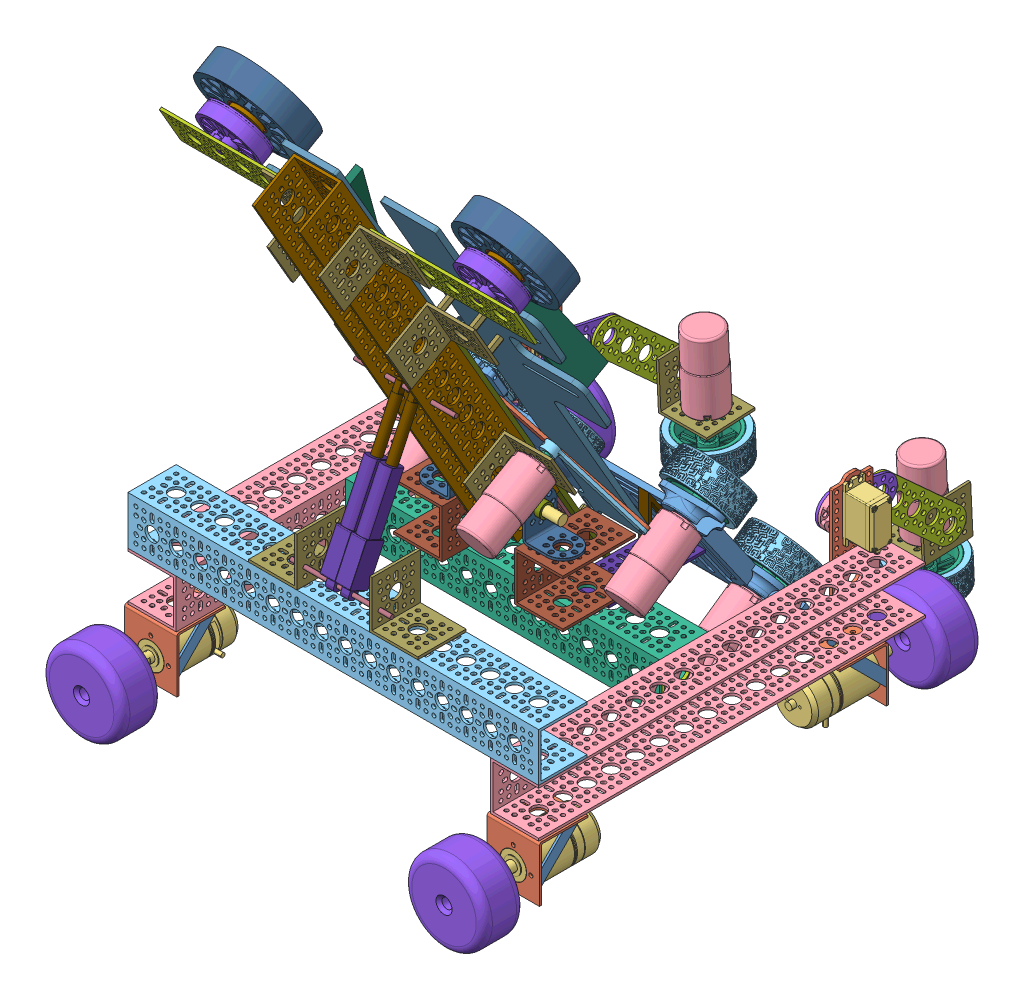
SolidWorks assembly 底座3.0, configuration 默认. Lengths in mm. (continued)
Mates (geometry in assembly coordinates): (continued)
- Concentric428: concentric anti-aligned: cylinder of 连杆02-1 through (57.5295 256.5301 499.31) axis (0 -0.499817 0.866131) radius 1.6; cylinder of 连杆01-5 through (57.5295 253.6311 504.3336) axis (0 0.499817 -0.866131) radius 1.6
- Concentric437: concentric aligned: cylinder of 5孔平板-1 through (85.3414 565.4353 686.9217) axis (0 -0.499817 0.866131) radius 7; cylinder of 发射无刷电机-1 through (85.3414 563.8859 689.6067) axis (0 -0.499817 0.866131) radius 12.5
- Coincident197: coincident anti-aligned: plane of 5孔平板-1 through (-10.6586 580.3085 704.1637) normal (0 0.499817 -0.866131); plane of 发射无刷电机-1 through (85.3414 561.6867 693.4176) normal (0 -0.499817 0.866131)
- Concentric438: concentric aligned: cylinder of 发射无刷电机-1 through (85.3414 578.5805 664.1424) axis (0 -0.499817 0.866131) radius 2; cylinder of 发射法兰-1 through (85.3414 578.0807 665.0086) axis (0 -0.499817 0.866131) radius 2.15
- Tangent7: tangent anti-aligned: plane of 5孔平板-1 through (87.3414 579.2934 694.9187) normal (-1 0 0); cylinder of 发射无刷电机-1 through (86.1414 574.6903 695.8416) axis (0 -0.499817 0.866131) radius 1.2
- Coincident198: coincident anti-aligned: plane of 发射无刷电机-1 through (94.8219 575.055 669.0353) normal (0 0.499817 -0.866131); plane of 发射法兰-1 through (85.3414 575.5816 669.3392) normal (0 -0.499817 0.866131)
- Concentric439: concentric anti-aligned: cylinder of 发射无刷电机-1 through (85.7254 577.7689 677.5287) axis (0 0.499817 -0.866131) radius 1.2; cylinder of 发射法兰-1 through (85.7254 583.2668 668.0013) axis (0 -0.499817 0.866131) radius 1.6
- Concentric440: concentric aligned: cylinder of 发射法兰-1 through (85.3414 581.0796 659.8118) axis (0 -0.499817 0.866131) radius 9.5; cylinder of 摩擦轮-2/摩擦轮.STEP-1/3613-0014-0096 Core.STEP-1 through (85.3414 581.0796 659.8118) axis (0 -0.499817 0.866131) radius 7
- Coincident199: coincident anti-aligned: plane of 发射法兰-1 through (85.3414 581.0796 659.8118) normal (0 0.499817 -0.866131); plane of 摩擦轮-2/摩擦轮.STEP-1/3613-0014-0096 Core.STEP-1 through (85.3414 581.0796 659.8118) normal (0 -0.499817 0.866131)
- Concentric441: concentric anti-aligned: cylinder of 发射法兰-1 through (74.0508 580.2073 662.7721) axis (0 0.499817 -0.866131) radius 2.1; cylinder of 摩擦轮-2/摩擦轮.STEP-1/3613-0014-0096 Core.STEP-1 through (74.0508 581.7068 660.1737) axis (0 -0.499817 0.866131) radius 2
- Coincident200: coincident anti-aligned: plane of 432mm-U型梁-1 through (-18.6586 602.8059 766.2151) normal (1 0 0); plane of 48x48-L形支架-1 through (-18.6586 557.2331 749.1529) normal (-1 0 0)
- Concentric442: concentric anti-aligned: cylinder of 432mm-U型梁-1 through (-28.6586 549.5096 698.5135) axis (1 0 0) radius 2; cylinder of 48x48-L形支架-1 through (-8.6586 549.5096 698.5135) axis (-1 0 0) radius 2
- Concentric443: concentric anti-aligned: cylinder of 432mm-U型梁-1 through (-28.6586 563.3677 706.5106) axis (1 0 0) radius 2; cylinder of 48x48-L形支架-1 through (-8.6586 563.3677 706.5106) axis (-1 0 0) radius 2
- Concentric444: concentric anti-aligned: cylinder of 48x48-L形支架-1 through (21.3414 569.2971 712.2414) axis (0 0.499817 -0.866131) radius 2; cylinder of 5孔平板-1 through (21.3414 579.2934 694.9187) axis (0 -0.499817 0.866131) radius 2
- Concentric445: concentric anti-aligned: cylinder of 48x48-L形支架-1 through (21.3414 541.5809 696.2472) axis (0 0.499817 -0.866131) radius 2; cylinder of 5孔平板-1 through (21.3414 551.5772 678.9246) axis (0 -0.499817 0.866131) radius 2
- Coincident202: coincident anti-aligned: plane of 发射法兰-2 through (-170.6586 575.5816 669.3392) normal (0 -0.499817 0.866131); plane of 发射无刷电机-3 through (-180.1392 576.1082 669.6431) normal (0 0.499817 -0.866131)
- Tangent9: tangent anti-aligned: cylinder of 发射无刷电机-3 through (-171.4586 553.0815 683.3718) axis (0 -0.499817 0.866131) radius 1.2; plane of 5孔平板-3 through (-172.6586 551.5772 678.9246) normal (1 0 0)
- Concentric446: concentric aligned: cylinder of 发射法兰-2 through (-170.6586 578.0807 665.0086) axis (0 -0.499817 0.866131) radius 2.15; cylinder of 发射无刷电机-3 through (-170.6586 578.5805 664.1424) axis (0 -0.499817 0.866131) radius 2
- Concentric447: concentric anti-aligned: cylinder of 发射法兰-2 through (-171.0426 572.8946 662.0158) axis (0 -0.499817 0.866131) radius 1.6; cylinder of 发射无刷电机-3 through (-171.0426 567.3966 671.5432) axis (0 0.499817 -0.866131) radius 1.2
- Concentric448: concentric aligned: cylinder of 摩擦轮-3/摩擦轮.STEP-1/3613-0014-0096 Core.STEP-1 through (-170.6586 581.0796 659.8118) axis (0 -0.499817 0.866131) radius 7; cylinder of 发射法兰-2 through (-170.6586 581.0796 659.8118) axis (0 -0.499817 0.866131) radius 9.5
- Concentric449: concentric anti-aligned: cylinder of 摩擦轮-3/摩擦轮.STEP-1/3613-0014-0096 Core.STEP-1 through (-159.3681 580.4525 659.4499) axis (0 -0.499817 0.866131) radius 2; cylinder of 发射法兰-2 through (-159.3681 578.953 662.0483) axis (0 0.499817 -0.866131) radius 2.1
- Coincident203: coincident anti-aligned: plane of 摩擦轮-3/摩擦轮.STEP-1/3613-0014-0096 Core.STEP-1 through (-170.6586 581.0796 659.8118) normal (0 -0.499817 0.866131); plane of 发射法兰-2 through (-170.6586 581.0796 659.8118) normal (0 0.499817 -0.866131)
- Concentric450: concentric anti-aligned: cylinder of 5孔平板-3 through (-106.6586 579.2934 694.9187) axis (0 -0.499817 0.866131) radius 2; cylinder of 48x48-L形支架-13 through (-106.6586 569.2971 712.2414) axis (0 0.499817 -0.866131) radius 2
- Concentric451: concentric anti-aligned: cylinder of 5孔平板-3 through (-106.6586 551.5772 678.9246) axis (0 -0.499817 0.866131) radius 2; cylinder of 48x48-L形支架-13 through (-106.6586 541.5809 696.2472) axis (0 0.499817 -0.866131) radius 2
- Coincident205: coincident anti-aligned: plane of 发射无刷电机-3 through (-170.6586 561.6867 693.4176) normal (0 -0.499817 0.866131); plane of 5孔平板-3 through (-74.6586 543.0649 682.6716) normal (0 0.499817 -0.866131)
- Concentric452: concentric aligned: cylinder of 发射无刷电机-3 through (-170.6586 563.8859 689.6067) axis (0 -0.499817 0.866131) radius 12.5; cylinder of 5孔平板-3 through (-170.6586 565.4353 686.9217) axis (0 -0.499817 0.866131) radius 7
- Coincident206: coincident anti-aligned: plane of 432mm-U型梁-1 through (-66.6586 602.8059 766.2151) normal (-1 0 0); plane of 48x48-L形支架-13 through (-66.6586 515.6588 725.1616) normal (1 0 0)
- Concentric453: concentric anti-aligned: cylinder of 432mm-U型梁-1 through (-56.6586 570.2967 710.5091) axis (-1 0 0) radius 2; cylinder of 48x48-L形支架-13 through (-76.6586 570.2967 710.5091) axis (1 0 0) radius 2
- Concentric454: concentric anti-aligned: cylinder of 432mm-U型梁-1 through (-56.6586 542.5805 694.5149) axis (-1 0 0) radius 2; cylinder of 48x48-L形支架-13 through (-76.6586 542.5805 694.5149) axis (1 0 0) radius 2
- Concentric455: concentric anti-aligned: cylinder of 432mm-U型梁-1 through (-28.6586 448.5044 649.463) axis (1 0 0) radius 7; cylinder of 48x48-L形支架-14 through (-8.6586 448.5044 649.463) axis (-1 0 0) radius 7
- Coincident207: coincident anti-aligned: plane of 432mm-U型梁-1 through (-18.6586 602.8059 766.2151) normal (1 0 0); plane of 48x48-L形支架-14 through (-18.6586 457.2959 682.2457) normal (-1 0 0)
- Concentric456: concentric anti-aligned: cylinder of 432mm-U型梁-1 through (-28.6586 442.6434 627.6078) axis (1 0 0) radius 2; cylinder of 48x48-L形支架-14 through (-8.6586 442.6434 627.6078) axis (-1 0 0) radius 2
- Coincident208: coincident anti-aligned: plane of 432mm-U型梁-1 through (-66.6586 602.8059 766.2151) normal (-1 0 0); plane of 48x48-L形支架-15 through (-66.6586 415.7216 658.2545) normal (1 0 0)
- Concentric457: concentric anti-aligned: cylinder of 432mm-U型梁-1 through (-56.6586 448.5044 649.463) axis (-1 0 0) radius 7; cylinder of 48x48-L形支架-15 through (-76.6586 448.5044 649.463) axis (1 0 0) radius 7
- Concentric458: concentric anti-aligned: cylinder of 432mm-U型梁-1 through (-56.6586 470.3596 643.602) axis (-1 0 0) radius 2; cylinder of 48x48-L形支架-15 through (-76.6586 470.3596 643.602) axis (1 0 0) radius 2
- Concentric459: concentric anti-aligned: cylinder of 48x48-L形支架-14 through (21.3414 469.3599 645.3342) axis (0 0.499817 -0.866131) radius 2; cylinder of 铜柱-1 through (21.3414 481.8554 623.6809) axis (0 -0.499817 0.866131) radius 1.6
- Coincident209: coincident anti-aligned: plane of 48x48-L形支架-14 through (-18.6586 481.2871 640.6714) normal (0 0.499817 -0.866131); plane of 铜柱-1 through (21.3414 474.3581 636.6729) normal (0 -0.499817 0.866131)
- Concentric460: concentric anti-aligned: cylinder of 48x48-L形支架-14 through (21.3414 441.6437 629.3401) axis (0 0.499817 -0.866131) radius 2; cylinder of 铜柱-2 through (21.3414 454.1392 607.6868) axis (0 -0.499817 0.866131) radius 1.6
- Coincident210: coincident anti-aligned: plane of 48x48-L形支架-14 through (-18.6586 481.2871 640.6714) normal (0 0.499817 -0.866131); plane of 铜柱-2 through (21.3414 446.6419 620.6788) normal (0 -0.499817 0.866131)
- Concentric461: concentric anti-aligned: cylinder of 48x48-L形支架-14 through (-10.6586 469.3599 645.3342) axis (0 0.499817 -0.866131) radius 2; cylinder of 铜柱-3 through (-10.6586 481.8554 623.6809) axis (0 -0.499817 0.866131) radius 1.6
- Coincident211: coincident anti-aligned: plane of 48x48-L形支架-14 through (-18.6586 481.2871 640.6714) normal (0 0.499817 -0.866131); plane of 铜柱-3 through (-10.6586 474.3581 636.6729) normal (0 -0.499817 0.866131)
- Concentric462: concentric anti-aligned: cylinder of 48x48-L形支架-15 through (-106.6586 441.6437 629.3401) axis (0 0.499817 -0.866131) radius 2; cylinder of 铜柱-6 through (-106.6586 454.1392 607.6868) axis (0 -0.499817 0.866131) radius 1.6
- Concentric463: concentric anti-aligned: cylinder of 48x48-L形支架-15 through (-106.6586 469.3599 645.3342) axis (0 0.499817 -0.866131) radius 2; cylinder of 铜柱-5 through (-106.6586 481.8554 623.6809) axis (0 -0.499817 0.866131) radius 1.6
- Concentric464: concentric anti-aligned: cylinder of 48x48-L形支架-15 through (-74.6586 469.3599 645.3342) axis (0 0.499817 -0.866131) radius 2; cylinder of 铜柱-4 through (-74.6586 481.8554 623.6809) axis (0 -0.499817 0.866131) radius 1.6
- Coincident212: coincident anti-aligned: plane of 48x48-L形支架-15 through (-66.6586 439.7129 616.6802) normal (0 0.499817 -0.866131); plane of 铜柱-6 through (-106.6586 446.6419 620.6788) normal (0 -0.499817 0.866131)
- Coincident213: coincident anti-aligned: plane of 48x48-L形支架-15 through (-66.6586 439.7129 616.6802) normal (0 0.499817 -0.866131); plane of 铜柱-5 through (-106.6586 474.3581 636.6729) normal (0 -0.499817 0.866131)
- Coincident214: coincident anti-aligned: plane of 48x48-L形支架-15 through (-66.6586 439.7129 616.6802) normal (0 0.499817 -0.866131); plane of 铜柱-4 through (-74.6586 474.3581 636.6729) normal (0 -0.499817 0.866131)
- Concentric465: concentric anti-aligned: cylinder of 312mm-U型梁-2 through (105.3414 179.4201 533.5024) axis (0 1 0) radius 2; cone of 电机转向座-7 through (105.3414 186.9201 533.5024) axis (0 -1 0)
- Concentric466: concentric anti-aligned: cylinder of 312mm-U型梁-2 through (105.3414 179.4201 501.5024) axis (0 1 0) radius 2; cone of 电机转向座-7 through (105.3414 186.9201 501.5024) axis (0 -1 0)
- Concentric467: concentric anti-aligned: cylinder of 312mm-U型梁-2 through (105.3414 181.4201 531.5024) axis (0 0 1) radius 2; cone of 电机转向座-7 through (105.3414 181.4201 538.6524) axis (0 0 -1)
- Concentric468: concentric anti-aligned: cylinder of 312mm-U型梁-2 through (105.3414 149.4201 531.5024) axis (0 0 1) radius 2; cone of 电机转向座-7 through (105.3414 149.4201 538.6524) axis (0 0 -1)
- Concentric469: concentric anti-aligned: cylinder of 312mm-U型梁-2 through (-190.6586 179.4201 501.5024) axis (0 1 0) radius 2; cone of 电机转向座-8 through (-190.6586 186.9201 501.5024) axis (0 -1 0)
- Concentric470: concentric anti-aligned: cylinder of 312mm-U型梁-2 through (-190.6586 179.4201 533.5024) axis (0 1 0) radius 2; cone of 电机转向座-8 through (-190.6586 186.9201 533.5024) axis (0 -1 0)
- Concentric471: concentric anti-aligned: cylinder of 312mm-U型梁-2 through (-190.6586 181.4201 531.5024) axis (0 0 1) radius 2; cone of 电机转向座-8 through (-190.6586 181.4201 539.0024) axis (0 0 -1)
- Concentric472: concentric anti-aligned: cylinder of 312mm-U型梁-2 through (-190.6586 149.4201 531.5024) axis (0 0 1) radius 2; cone of 电机转向座-8 through (-190.6586 149.4201 539.0024) axis (0 0 -1)
- Concentric473: concentric aligned: cylinder of 384mm-U型梁-1 through (-208.6586 165.4201 517.5024) axis (1 0 0) radius 7; cylinder of 电机转向座-8 through (-198.6586 165.4201 517.5024) axis (1 0 0) radius 7
- Concentric474: concentric aligned: cylinder of 384mm-U型梁-1 through (-208.6586 149.4201 533.5024) axis (1 0 0) radius 2; cone of 电机转向座-8 through (-198.6586 149.4201 533.5024) axis (1 0 0)
- Coincident215: coincident anti-aligned: plane of 384mm-U型梁-1 through (-198.6586 141.4201 325.5024) normal (1 0 0); plane of 电机转向座-8 through (-198.6586 165.4201 517.5024) normal (-1 0 0)
- Concentric476: concentric aligned: cylinder of 432mm-U型梁-1 through (-26.6586 254.5595 521.3795) axis (0 0.499817 -0.866131) radius 2; cylinder of 2孔平板-6 through (-26.6586 253.3099 523.5448) axis (0 0.499817 -0.866131) radius 2
- Concentric477: concentric aligned: cylinder of 432mm-U型梁-1 through (-58.6586 254.5595 521.3795) axis (0 0.499817 -0.866131) radius 2; cylinder of 2孔平板-6 through (-58.6586 253.3099 523.5448) axis (0 0.499817 -0.866131) radius 2
- Coincident216: coincident anti-aligned: plane of 432mm-U型梁-1 through (-21.1586 625.5476 726.8061) normal (0 -0.499817 0.866131); plane of 2孔平板-6 through (-18.6586 265.2372 518.8821) normal (0 0.499817 -0.866131)
- Concentric478: concentric anti-aligned: cylinder of 2孔平板-6 through (-26.6586 204.8066 495.555) axis (0 0.499817 -0.866131) radius 2; cylinder of 铜柱-7 through (-26.6586 217.3021 473.9018) axis (0 -0.499817 0.866131) radius 1.6
- Concentric479: concentric anti-aligned: cylinder of 2孔平板-6 through (-58.6586 204.8066 495.555) axis (0 0.499817 -0.866131) radius 2; cylinder of 铜柱-8 through (-58.6586 217.3021 473.9018) axis (0 -0.499817 0.866131) radius 1.6
- Coincident217: coincident anti-aligned: plane of 2孔平板-6 through (-18.6586 265.2372 518.8821) normal (0 0.499817 -0.866131); plane of 铜柱-7 through (-26.6586 209.8048 486.8937) normal (0 -0.499817 0.866131)
- Coincident218: coincident anti-aligned: plane of 2孔平板-6 through (-18.6586 265.2372 518.8821) normal (0 0.499817 -0.866131); plane of 铜柱-8 through (-58.6586 209.8048 486.8937) normal (0 -0.499817 0.866131)
- Coincident219: coincident anti-aligned: plane of 铜柱-3 through (-10.6586 481.8554 623.6809) normal (0 0.499817 -0.866131); plane of 小兔侧板-1 through (-20.6586 476.6586 620.682) normal (0 -0.499817 0.866131)
- Concentric480: concentric aligned: cylinder of 铜柱-3 through (-10.6586 481.8554 623.6809) axis (0 -0.499817 0.866131) radius 1.6; cylinder of 小兔侧板-1 through (-10.6586 484.3544 619.3503) axis (0 -0.499817 0.866131) radius 2
- Concentric481: concentric aligned: cylinder of 铜柱-1 through (21.3414 481.8554 623.6809) axis (0 -0.499817 0.866131) radius 1.6; cylinder of 小兔侧板-1 through (21.3414 484.3544 619.3503) axis (0 -0.499817 0.866131) radius 2
- Distance14: distance = 28 mm aligned: plane of 升降轴-2 through (-94.6586 392.004 635.3313) normal (-1 0 0); plane of 432mm-U型梁-1 through (-66.6586 602.8059 766.2151) normal (-1 0 0)
- Coincident220: coincident anti-aligned: plane of 48x48-L形支架-1 through (-18.6586 581.2243 707.5786) normal (0 0.499817 -0.866131); plane of 5孔平板-1 through (-10.6586 539.65 683.5874) normal (0 -0.499817 0.866131)
- Coincident221: coincident anti-aligned: plane of 5孔平板-3 through (-74.6586 581.2243 707.5786) normal (0 -0.499817 0.866131); plane of 48x48-L形支架-13 through (-66.6586 539.65 683.5874) normal (0 0.499817 -0.866131)
- Concentric482: concentric anti-aligned: cylinder of 铜柱-5 through (-106.6586 481.8554 623.6809) axis (0 -0.499817 0.866131) radius 1.6; cylinder of 小兔侧板-2 through (-106.6586 481.8554 623.6809) axis (0 0.499817 -0.866131) radius 2
- Concentric483: concentric anti-aligned: cylinder of 铜柱-4 through (-74.6586 481.8554 623.6809) axis (0 -0.499817 0.866131) radius 1.6; cylinder of 小兔侧板-2 through (-74.6586 481.8554 623.6809) axis (0 0.499817 -0.866131) radius 2
- Coincident222: coincident anti-aligned: plane of 铜柱-5 through (-106.6586 481.8554 623.6809) normal (0 0.499817 -0.866131); plane of 小兔侧板-2 through (-64.6586 476.6586 620.682) normal (0 -0.499817 0.866131)
- Coincident223: coincident anti-aligned: plane of 小兔侧板-1 through (-20.6586 479.1577 616.3514) normal (0 0.499817 -0.866131); plane of 滚针版-1 through (68.7015 414.8521 579.2426) normal (0 -0.499817 0.866131)
- Distance15: distance = 10 mm: line of 滚针版-1 through (24.3414 520.6909 640.3189) axis (0 0.499817 -0.866131); line of 小兔侧板-1 through (34.3414 590.0224 680.328) axis (0 -0.866131 -0.499817)
- Distance16: distance = 20 mm: line of 滚针版-1 through (74.3414 432.1197 553.4159) axis (0 -0.499817 0.866131); line of 小兔侧板-1 through (94.3414 435.8511 591.3605) axis (0 -0.866131 -0.499817)
- Distance17: distance = 0 mm: line of 小兔侧板-1 through (44.3414 522.4642 641.3423) axis (1 0 0); line of 滚针版-1 through (29.9812 522.4642 641.3423) axis (0 0.499817 -0.866131)
- Coincident224: coincident anti-aligned: plane of 小兔侧板-2 through (-64.6586 479.1577 616.3514) normal (0 0.499817 -0.866131); plane of 滚针版-2 through (-159.6586 416.6254 580.2659) normal (0 -0.499817 0.866131)
- Distance18: distance = 10 mm: line of 小兔侧板-2 through (-119.6586 590.0224 680.328) axis (0 -0.866131 -0.499817); line of 滚针版-2 through (-109.6586 520.6909 640.3189) axis (0 0.499817 -0.866131)
- Distance19: distance = 20 mm: line of 滚针版-2 through (-159.6586 432.1197 553.4159) axis (0 -0.499817 0.866131); line of 小兔侧板-2 through (-179.6586 435.8511 591.3605) axis (0 -0.866131 -0.499817)
- Distance20: distance = 0 mm: line of 滚针版-2 through (-115.2985 522.4642 641.3423) axis (0 0.499817 -0.866131); line of 小兔侧板-2 through (-129.6586 522.4642 641.3423) axis (-1 0 0)
- Concentric484: concentric: cylinder of 432mm-U型梁-1 through (-26.6586 254.5595 521.3795) axis (0 0.499817 -0.866131) radius 2; cylinder of 抓钩滑轨-1 through (-26.6586 183.3382 468.7342) axis (0 0.499817 -0.866131) radius 2
- Coincident225: coincident: plane of 432mm-U型梁-1 through (-66.6586 626.7971 724.6408) normal (0 0.499817 -0.866131); plane of 抓钩滑轨-1 through (-19.1586 167.7478 459.7375) normal (0 -0.499817 0.866131)
- Concentric485: concentric: cylinder of 432mm-U型梁-1 through (-26.6586 413.9276 613.3459) axis (0 0.499817 -0.866131) radius 2; cylinder of 抓钩滑轨-1 through (-26.6586 418.9257 604.6846) axis (0 0.499817 -0.866131) radius 2
- Concentric486: concentric: cylinder of 432mm-U型梁-1 through (-58.6586 413.9276 613.3459) axis (0 0.499817 -0.866131) radius 2; cylinder of 抓钩滑轨-2 through (-58.6586 418.9257 604.6846) axis (0 0.499817 -0.866131) radius 2
- Concentric487: concentric: cylinder of 432mm-U型梁-1 through (-58.6586 254.5595 521.3795) axis (0 0.499817 -0.866131) radius 2; cylinder of 抓钩滑轨-2 through (-58.6586 183.3382 468.7342) axis (0 0.499817 -0.866131) radius 2
- Coincident226: coincident: plane of 432mm-U型梁-1 through (-66.6586 626.7971 724.6408) normal (0 0.499817 -0.866131); plane of 抓钩滑轨-2 through (-51.1586 167.7478 459.7375) normal (0 -0.499817 0.866131)
- Coincident227: coincident anti-aligned: plane of 312mm-U型梁-2 through (-198.6586 186.9201 539.0024) normal (0 -1 0); plane of 3孔平板-1 through (38.8414 186.9201 517.5024) normal (0 1 0)
- Concentric488: concentric aligned: cylinder of 72mm-U型梁-1 through (33.3414 199.4201 509.5024) axis (0 -1 0) radius 2; cylinder of 3孔平板-1 through (33.3414 194.4201 509.5024) axis (0 -1 0) radius 2
- Concentric489: concentric aligned: cylinder of 72mm-U型梁-1 through (1.3414 199.4201 509.5024) axis (0 -1 0) radius 2; cylinder of 3孔平板-1 through (1.3414 194.4201 509.5024) axis (0 -1 0) radius 2
- Coincident228: coincident anti-aligned: plane of 3孔平板-1 through (38.8414 186.9201 517.5024) normal (0 1 0); plane of 03铲板支架-1 through (-3.6586 186.9201 413.9931) normal (0 -1 0)
- Concentric490: concentric aligned: cylinder of 3孔平板-1 through (1.3414 194.4201 429.5024) axis (0 -1 0) radius 2; cylinder of 03铲板支架-1 through (1.3414 189.9201 429.5024) axis (0 -1 0) radius 2
- Concentric491: concentric aligned: cylinder of 3孔平板-1 through (1.3414 194.4201 437.5024) axis (0 -1 0) radius 2; cylinder of 03铲板支架-1 through (1.3414 189.9201 437.5024) axis (0 -1 0) radius 2
- Coincident229: coincident anti-aligned: plane of 03铲板支架-1 through (-3.6586 231.9201 445.5024) normal (0 0.573576 -0.819152); plane of 铲板-1 through (52.3414 232.7164 446.06) normal (0 -0.573576 0.819152)
- Parallel12: parallel anti-aligned: line of 312mm-U型梁-2 through (-198.6586 189.4201 493.5024) axis (1 0 0); line of 铲板-1 through (52.3414 73.0356 316.0571) axis (-1 0 0)
- Tangent10: tangent: cylinder of 麦轮（临时）-2 through (137.3414 109.4201 284.5024) axis (0 0 1) radius 40; line of 铲板-1 through (52.3414 69.4201 319.5109) axis (-1 0 0)
- Distance21: distance = 61 mm anti-aligned: plane of 384mm-U型梁-2 through (113.3414 189.4201 325.5024) normal (-1 0 0); plane of 铲板-1 through (52.3414 124.5662 327.6053) normal (1 0 0)
- Concentric492: concentric aligned: cylinder of 384mm-U型梁-2 through (123.3414 165.4201 349.5024) axis (-1 0 0) radius 7; cylinder of 舵机支架-1 through (176.5948 165.4201 349.5024) axis (-1 0 0) radius 7
- Coincident230: coincident anti-aligned: plane of 384mm-U型梁-2 through (113.3414 189.4201 325.5024) normal (-1 0 0); plane of 舵机支架-1 through (113.3414 223.4201 349.5024) normal (1 0 0)
- Concentric493: concentric aligned: cylinder of 384mm-U型梁-2 through (123.3414 181.4201 333.5024) axis (-1 0 0) radius 2; cylinder of 舵机支架-1 through (113.3414 181.4201 333.5024) axis (-1 0 0) radius 2
- Coincident231: coincident anti-aligned: plane of 舵机支架-1 through (113.3414 223.4201 349.5024) normal (1 0 0); plane of 舵机-1 through (113.3414 249.0701 340.9524) normal (-1 0 0)
- Parallel13: parallel anti-aligned: plane of 舵机支架-1 through (110.3414 223.4201 347.5024) normal (0 0 1); plane of 舵机-1 through (116.0414 223.4201 348.8274) normal (0 0 -1)
- Distance23: distance = 1.325 mm anti-aligned: plane of 舵机-1 through (116.0414 223.4201 348.8274) normal (0 0 -1); plane of 舵机支架-1 through (110.3414 223.4201 347.5024) normal (0 0 1)
- Distance24: distance = 1.75 mm anti-aligned: plane of 舵机-1 through (107.4414 203.5701 358.9524) normal (0 -1 0); plane of 舵机支架-1 through (113.5121 201.8201 349.5024) normal (0 1 0)
- Distance25: distance = 1.325 mm anti-aligned: plane of 舵机-2 through (-201.3586 223.4201 350.1774) normal (0 0 1); plane of 舵机支架-2 through (-195.6586 223.4201 351.5024) normal (0 0 -1)
- Coincident232: coincident anti-aligned: plane of 舵机支架-2 through (-198.6586 223.4201 349.5024) normal (-1 0 0); plane of 舵机-2 through (-198.6586 249.0701 358.0524) normal (1 0 0)
- Parallel14: parallel anti-aligned: plane of 舵机支架-2 through (-195.6586 223.4201 351.5024) normal (0 0 -1); plane of 舵机-2 through (-201.3586 223.4201 350.1774) normal (0 0 1)
- Distance26: distance = 1.75 mm anti-aligned: plane of 舵机-2 through (-192.7586 203.5701 340.0524) normal (0 -1 0); plane of 舵机支架-2 through (-198.8293 201.8201 349.5024) normal (0 1 0)
- Concentric496: concentric aligned: cylinder of 384mm-U型梁-1 through (-208.6586 165.4201 349.5024) axis (1 0 0) radius 7; cylinder of 舵机支架-2 through (-261.9121 165.4201 349.5024) axis (1 0 0) radius 7
- Coincident233: coincident anti-aligned: plane of 384mm-U型梁-1 through (-198.6586 141.4201 325.5024) normal (1 0 0); plane of 舵机支架-2 through (-198.6586 223.4201 349.5024) normal (-1 0 0)
- Concentric497: concentric aligned: cylinder of 384mm-U型梁-1 through (-208.6586 181.4201 333.5024) axis (1 0 0) radius 2; cylinder of 舵机支架-2 through (-198.6586 181.4201 333.5024) axis (1 0 0) radius 2
- Concentric498: concentric aligned: cone of 舵机-1 through (99.1414 213.5701 349.4524) axis (1 0 0); cylinder of 舵机法兰-1 through (49.3148 213.5701 349.4524) axis (1 0 0) radius 4.99
- Coincident234: coincident anti-aligned: plane of 舵机-1 through (99.1414 213.5701 349.4524) normal (-1 0 0); plane of 舵机法兰-1 through (99.1414 213.5701 349.4524) normal (1 0 0)
- Concentric499: concentric aligned: cone of 舵机-2 through (-184.4586 213.5701 349.5524) axis (-1 0 0); cylinder of 舵机法兰-2 through (-134.6321 213.5701 349.5524) axis (-1 0 0) radius 4.99
- Coincident235: coincident anti-aligned: plane of 舵机-2 through (-184.4586 213.5701 349.5524) normal (1 0 0); plane of 舵机法兰-2 through (-184.4586 213.5701 349.5524) normal (-1 0 0)
- Coincident247: coincident anti-aligned: plane of 一级摩擦轮电机01-6 through (-150.8586 120.7329 230.6107) normal (0 -0.998844 -0.048076); plane of 一级摩擦轮电机02-5 through (-150.8586 120.7329 230.6107) normal (0 0.998844 0.048076)
- Concentric514: concentric anti-aligned: cylinder of 一级摩擦轮电机01-6 through (-150.8586 120.7329 230.6107) axis (0 -0.998844 -0.048076) radius 4; cylinder of 一级摩擦轮电机02-5 through (-150.8586 100.7561 229.6491) axis (0 0.998844 0.048076) radius 4
- Concentric516: concentric aligned: cylinder of 一级摩擦轮电机02-5 through (-150.8586 100.7561 229.6491) axis (0 0.998844 0.048076) radius 4; cylinder of 蓝色橡胶轮胎-1/蓝色橡胶轮胎.stp-1/LUNGU2.stp-1 through (-150.8586 73.5875 228.3415) axis (0 0.998844 0.048076) radius 5.7
- Tangent13: tangent: line of 一级摩擦轮电机02-5 through (-148.2437 100.9016 226.6258) axis (-0.999948 -0.000491 0.010207); cylinder of 蓝色橡胶轮胎-1/蓝色橡胶轮胎.stp-1/LUNGU2.stp-1 through (-145.1644 102.3419 229.9827) axis (0.999078 -0.002064 0.042883) radius 1.6
- Concentric531: concentric anti-aligned: cylinder of 圆角孔板5孔-2 through (-177.3586 139.2115 231.5001) axis (1 0 0) radius 7; cylinder of 48x48-L形支架-16 through (-164.8586 139.2115 231.5001) axis (-1 0 0) radius 7
- Coincident256: coincident anti-aligned: plane of 圆角孔板5孔-2 through (-174.8586 203.7518 302.5673) normal (1 0 0); plane of 48x48-L形支架-16 through (-174.8586 114.0855 254.3185) normal (-1 0 0)
- Concentric532: concentric anti-aligned: cylinder of 一级摩擦轮电机01-6 through (-150.8586 117.7364 230.4664) axis (0 0.998844 0.048076) radius 11; cylinder of 48x48-L形支架-16 through (-150.8586 125.2277 230.827) axis (0 -0.998844 -0.048076) radius 7
- Coincident257: coincident anti-aligned: plane of 一级摩擦轮电机01-6 through (-150.8586 117.7364 230.4664) normal (0 -0.998844 -0.048076); plane of 48x48-L形支架-16 through (-172.3586 116.5826 254.4387) normal (0 0.998844 0.048076)
- Tangent14: tangent anti-aligned: cylinder of 一级摩擦轮电机01-6 through (-136.8676 125.052 230.318) axis (0 -0.998844 -0.048076) radius 1.5; plane of 48x48-L形支架-16 through (-172.3586 125.3239 228.8293) normal (0 -0.048076 0.998844)
- Concentric533: concentric aligned: cylinder of 圆角孔板5孔-2 through (-177.3586 150.5122 232.044) axis (1 0 0) radius 2; cylinder of 48x48-L形支架-16 through (-174.8586 150.5122 232.044) axis (1 0 0) radius 2
- Concentric534: concentric anti-aligned: cylinder of 舵机法兰-2 through (-207.6859 213.5701 349.5524) axis (1 0 0) radius 7.01; cylinder of 圆角孔板3孔-2 through (-177.3586 213.5701 349.5524) axis (-1 0 0) radius 7
- Concentric535: concentric aligned: cone of 舵机法兰-2 through (-180.2086 223.0374 355.7469) axis (-1 0 0); cylinder of 圆角孔板3孔-2 through (-177.3586 223.0374 355.7469) axis (-1 0 0) radius 2
- Coincident259: coincident anti-aligned: plane of 舵机法兰-2 through (-179.8586 213.5701 349.5524) normal (1 0 0); plane of 圆角孔板3孔-2 through (-179.8586 213.5701 349.5524) normal (-1 0 0)
- Concentric536: concentric anti-aligned: cylinder of 圆角孔板5孔-2 through (-177.3586 203.7518 302.5673) axis (1 0 0) radius 7; cylinder of 圆角孔板3孔-2 through (-177.3586 203.7518 302.5673) axis (-1 0 0) radius 7
- Coincident260: coincident anti-aligned: plane of 圆角孔板5孔-2 through (-177.3586 203.7518 302.5673) normal (-1 0 0); plane of 圆角孔板3孔-2 through (-177.3586 213.5701 349.5524) normal (1 0 0)
- Concentric537: concentric aligned: cylinder of 舵机法兰-1 through (122.3686 213.5701 349.4524) axis (-1 0 0) radius 7.01; cylinder of 圆角孔板3孔-3 through (94.5414 213.5701 349.4524) axis (-1 0 0) radius 7
- Concentric538: concentric anti-aligned: cone of 舵机法兰-1 through (94.8914 223.0186 355.6755) axis (1 0 0); cylinder of 圆角孔板3孔-3 through (94.5414 223.0186 355.6755) axis (-1 0 0) radius 2
- Concentric539: concentric anti-aligned: cylinder of 圆角孔板3孔-3 through (94.5414 203.8941 302.4378) axis (-1 0 0) radius 7; cylinder of 圆角孔板5孔-3 through (89.5414 203.8941 302.4378) axis (1 0 0) radius 7
- Coincident261: coincident anti-aligned: plane of 圆角孔板3孔-3 through (92.0414 213.5701 349.4524) normal (-1 0 0); plane of 圆角孔板5孔-3 through (92.0414 203.8941 302.4378) normal (1 0 0)
- Coincident262: coincident anti-aligned: plane of 一级摩擦轮电机02-6 through (65.5414 120.7329 230.6107) normal (0 0.998844 0.048076); plane of 一级摩擦轮电机01-7 through (65.5414 120.7329 230.6107) normal (0 -0.998844 -0.048076)
- Concentric540: concentric anti-aligned: cylinder of 一级摩擦轮电机02-6 through (65.5414 100.7561 229.6491) axis (0 0.998844 0.048076) radius 4; cylinder of 一级摩擦轮电机01-7 through (65.5414 120.7329 230.6107) axis (0 -0.998844 -0.048076) radius 4
- Concentric541: concentric anti-aligned: cylinder of 48x48-L形支架-17 through (65.5414 125.2277 230.827) axis (0 -0.998844 -0.048076) radius 7; cylinder of 一级摩擦轮电机01-7 through (65.5414 117.7364 230.4664) axis (0 0.998844 0.048076) radius 11
- Coincident263: coincident anti-aligned: plane of 48x48-L形支架-17 through (87.0414 118.8902 206.4942) normal (0 0.998844 0.048076); plane of 一级摩擦轮电机01-7 through (65.5414 117.7364 230.4664) normal (0 -0.998844 -0.048076)
- Tangent15: tangent anti-aligned: plane of 48x48-L形支架-17 through (87.0414 125.1316 232.8247) normal (0 0.048076 -0.998844); cylinder of 一级摩擦轮电机01-7 through (51.5503 125.0039 231.3168) axis (0 -0.998844 -0.048076) radius 1.5
- Concentric542: concentric aligned: cylinder of 圆角孔板5孔-3 through (89.5414 139.2115 231.5001) axis (1 0 0) radius 7; cylinder of 48x48-L形支架-17 through (79.5414 139.2115 231.5001) axis (1 0 0) radius 7
- Concentric543: concentric aligned: cylinder of 圆角孔板5孔-3 through (89.5414 139.2115 231.5001) axis (1 0 0) radius 7; cylinder of 48x48-L形支架-17 through (79.5414 139.2115 231.5001) axis (1 0 0) radius 7
- Coincident265: coincident anti-aligned: plane of 圆角孔板5孔-3 through (89.5414 203.8941 302.4378) normal (-1 0 0); plane of 48x48-L形支架-17 through (89.5414 116.3931 206.374) normal (1 0 0)
- Coincident266: coincident anti-aligned: plane of 舵机法兰-1 through (94.5414 213.5701 349.4524) normal (-1 0 0); plane of 圆角孔板3孔-3 through (94.5414 213.5701 349.4524) normal (1 0 0)
- Concentric544: concentric aligned: cylinder of 一级摩擦轮电机02-6 through (65.5414 100.7561 229.6491) axis (0 0.998844 0.048076) radius 4; cylinder of 蓝色橡胶轮胎-2/蓝色橡胶轮胎.stp-1/LUNGU2.stp-1 through (65.5414 73.5875 228.3415) axis (0 0.998844 0.048076) radius 5.7
- Tangent16: tangent: line of 一级摩擦轮电机02-6 through (68.1565 100.9016 226.6259) axis (-0.999948 -0.000488 0.010147); cylinder of 蓝色橡胶轮胎-2/蓝色橡胶轮胎.stp-1/LUNGU2.stp-1 through (71.2358 102.342 229.9787) axis (0.999108 -0.00203 0.042182) radius 1.6
- Coincident267: coincident aligned: plane of 48x48-L形支架-16 through (-172.3586 140.3654 207.5278) normal (0 0.048076 -0.998844); plane of 48x48-L形支架-17 through (87.0414 140.3654 207.5278) normal (0 0.048076 -0.998844)
- Coincident268: coincident aligned: plane of 48x48-L形支架-16 through (-126.8586 114.0855 254.3185) normal (0 -0.998844 -0.048076); plane of 48x48-L形支架-17 through (41.5414 116.3931 206.374) normal (0 -0.998844 -0.048076)
- Lock1: lock: 
- Lock2: lock: 
- Tangent17: tangent anti-aligned: cylinder of 麦轮（临时）-1 through (-222.6586 109.4201 284.5024) axis (0 0 1) radius 40; cylinder of 铲板-1 through (102.3414 68.9201 319.3) axis (-1 0 0) radius 0.5
- Concentric549: concentric aligned: cylinder of 铲板-1 through (-152.6586 165.7822 384.7417) axis (0 -0.573576 0.819152) radius 9; cylinder of 一级摩擦轮电机01-8 through (-152.6586 153.257 402.6296) axis (0 -0.573576 0.819152) radius 11
- Coincident271: coincident anti-aligned: plane of 铲板-1 through (-152.6586 153.257 402.6296) normal (0 -0.573576 0.819152); plane of 一级摩擦轮电机01-8 through (-152.6586 153.257 402.6296) normal (0 0.573576 -0.819152)
- Coincident272: coincident anti-aligned: plane of 一级摩擦轮电机01-8 through (-152.6586 151.5363 405.0871) normal (0 0.573576 -0.819152); plane of 一级摩擦轮电机02-7 through (-152.6586 151.5363 405.0871) normal (0 -0.573576 0.819152)
- Concentric550: concentric anti-aligned: cylinder of 一级摩擦轮电机01-8 through (-152.6586 151.5363 405.0871) axis (0 0.573576 -0.819152) radius 4; cylinder of 一级摩擦轮电机02-7 through (-152.6586 163.0078 388.704) axis (0 -0.573576 0.819152) radius 4
- Concentric551: concentric aligned: cylinder of 一级摩擦轮电机02-7 through (-152.6586 163.0078 388.704) axis (0 -0.573576 0.819152) radius 4; cylinder of 蓝色橡胶轮胎-3/蓝色橡胶轮胎.stp-1/LUNGU2.stp-1 through (-152.6586 162.9504 388.786) axis (0 -0.573576 0.819152) radius 2.5
- Tangent18: tangent: circle of 一级摩擦轮电机02-7; cylinder of 蓝色橡胶轮胎-3/蓝色橡胶轮胎.stp-1/LUNGU2.stp-1 through (-147.6539 164.3248 391.5794) axis (0.876999 0.393596 0.275599) radius 1.6
- Concentric552: concentric aligned: cylinder of 铲板-1 through (67.3414 165.7822 384.7417) axis (0 -0.573576 0.819152) radius 9; cylinder of 一级摩擦轮电机01-9 through (67.3414 153.257 402.6296) axis (0 -0.573576 0.819152) radius 11
- Coincident273: coincident anti-aligned: plane of 铲板-1 through (67.3414 153.257 402.6296) normal (0 -0.573576 0.819152); plane of 一级摩擦轮电机01-9 through (67.3414 153.257 402.6296) normal (0 0.573576 -0.819152)
- Concentric553: concentric anti-aligned: cylinder of 铲板-1 through (67.3414 177.2504 392.7718) axis (0 -0.573576 0.819152) radius 1.6; cylinder of 一级摩擦轮电机01-9 through (67.3414 160.538 416.6395) axis (0 0.573576 -0.819152) radius 1.5
- Concentric554: concentric anti-aligned: cylinder of 铲板-1 through (-152.6586 177.2504 392.7718) axis (0 -0.573576 0.819152) radius 1.6; cylinder of 一级摩擦轮电机01-8 through (-152.6586 160.538 416.6395) axis (0 0.573576 -0.819152) radius 1.5
- Concentric555: concentric aligned: cylinder of 铲板-1 through (67.3414 264.0805 453.5709) axis (0 -0.573576 0.819152) radius 9; cylinder of 一级摩擦轮电机01-10 through (67.3414 251.5552 471.4588) axis (0 -0.573576 0.819152) radius 11
- Coincident274: coincident anti-aligned: plane of 铲板-1 through (67.3414 153.257 402.6296) normal (0 -0.573576 0.819152); plane of 一级摩擦轮电机01-10 through (67.3414 251.5552 471.4588) normal (0 0.573576 -0.819152)
- Concentric556: concentric anti-aligned: cylinder of 铲板-1 through (67.3414 275.5486 461.601) axis (0 -0.573576 0.819152) radius 1.6; cylinder of 一级摩擦轮电机01-10 through (67.3414 258.8363 485.4687) axis (0 0.573576 -0.819152) radius 1.5
- Coincident275: coincident anti-aligned: plane of 铲板-1 through (-152.6586 153.257 402.6296) normal (0 -0.573576 0.819152); plane of 一级摩擦轮电机01-11 through (-152.6586 251.5552 471.4588) normal (0 0.573576 -0.819152)
- Concentric557: concentric aligned: cylinder of 铲板-1 through (-152.6586 264.0805 453.5709) axis (0 -0.573576 0.819152) radius 9; cylinder of 一级摩擦轮电机01-11 through (-152.6586 251.5552 471.4588) axis (0 -0.573576 0.819152) radius 11
- Concentric558: concentric anti-aligned: cylinder of 铲板-1 through (-152.6586 275.5486 461.601) axis (0 -0.573576 0.819152) radius 1.6; cylinder of 一级摩擦轮电机01-11 through (-152.6586 258.8363 485.4687) axis (0 0.573576 -0.819152) radius 1.5
- Coincident276: coincident anti-aligned: plane of 一级摩擦轮电机01-11 through (-152.6586 249.8345 473.9162) normal (0 0.573576 -0.819152); plane of 一级摩擦轮电机02-8 through (-152.6586 249.8345 473.9162) normal (0 -0.573576 0.819152)
- Concentric559: concentric anti-aligned: cylinder of 一级摩擦轮电机01-11 through (-152.6586 249.8345 473.9162) axis (0 0.573576 -0.819152) radius 4; cylinder of 一级摩擦轮电机02-8 through (-152.6586 261.306 457.5332) axis (0 -0.573576 0.819152) radius 4
- Concentric560: concentric aligned: cylinder of 蓝色橡胶轮胎-4/蓝色橡胶轮胎.stp-1/LUNGU2.stp-1 through (-152.6586 261.2487 457.6151) axis (0 -0.573576 0.819152) radius 2.5; cylinder of 一级摩擦轮电机02-8 through (-152.6586 261.306 457.5332) axis (0 -0.573576 0.819152) radius 4
- Tangent19: tangent: cylinder of 蓝色橡胶轮胎-4/蓝色橡胶轮胎.stp-1/LUNGU2.stp-1 through (-158.0483 258.8686 457.7797) axis (-0.944846 -0.268284 -0.187855) radius 1.6; circle of 一级摩擦轮电机02-8
- Coincident277: coincident anti-aligned: plane of 一级摩擦轮电机01-9 through (67.3414 151.5363 405.0871) normal (0 0.573576 -0.819152); plane of 一级摩擦轮电机02-10 through (67.3414 151.5363 405.0871) normal (0 -0.573576 0.819152)
- Concentric561: concentric anti-aligned: cylinder of 一级摩擦轮电机01-9 through (67.3414 151.5363 405.0871) axis (0 0.573576 -0.819152) radius 4; cylinder of 一级摩擦轮电机02-10 through (67.3414 163.0078 388.704) axis (0 -0.573576 0.819152) radius 4
- Concentric562: concentric aligned: cylinder of 蓝色橡胶轮胎-5/蓝色橡胶轮胎.stp-1/LUNGU2.stp-1 through (67.3414 162.9504 388.786) axis (0 -0.573576 0.819152) radius 2.5; cylinder of 一级摩擦轮电机02-10 through (67.3414 163.0078 388.704) axis (0 -0.573576 0.819152) radius 4
- Tangent20: tangent: cylinder of 蓝色橡胶轮胎-5/蓝色橡胶轮胎.stp-1/LUNGU2.stp-1 through (61.8155 163.2353 390.8166) axis (-0.96998 0.199206 0.139485) radius 1.6; line of 一级摩擦轮电机02-10 through (67.1092 159.7367 386.4136) axis (0.787123 0.50525 0.35378)
- Coincident278: coincident anti-aligned: plane of 一级摩擦轮电机01-10 through (67.3414 249.8345 473.9162) normal (0 0.573576 -0.819152); plane of 一级摩擦轮电机02-9 through (67.3414 249.8345 473.9162) normal (0 -0.573576 0.819152)
- Concentric563: concentric anti-aligned: cylinder of 一级摩擦轮电机01-10 through (67.3414 249.8345 473.9162) axis (0 0.573576 -0.819152) radius 4; cylinder of 一级摩擦轮电机02-9 through (67.3414 261.306 457.5332) axis (0 -0.573576 0.819152) radius 4
- Concentric564: concentric aligned: cylinder of 蓝色橡胶轮胎-6/蓝色橡胶轮胎.stp-1/LUNGU2.stp-1 through (67.3414 261.2487 457.6151) axis (0 -0.573576 0.819152) radius 2.5; cylinder of 一级摩擦轮电机02-9 through (67.3414 261.306 457.5332) axis (0 -0.573576 0.819152) radius 4
- Tangent21: tangent: cylinder of 蓝色橡胶轮胎-6/蓝色橡胶轮胎.stp-1/LUNGU2.stp-1 through (62.0132 262.0472 460.0054) axis (-0.935521 0.289383 0.202628) radius 1.6; line of 一级摩擦轮电机02-9 through (67.1092 258.0349 455.2428) axis (0.787123 0.50525 0.35378)
